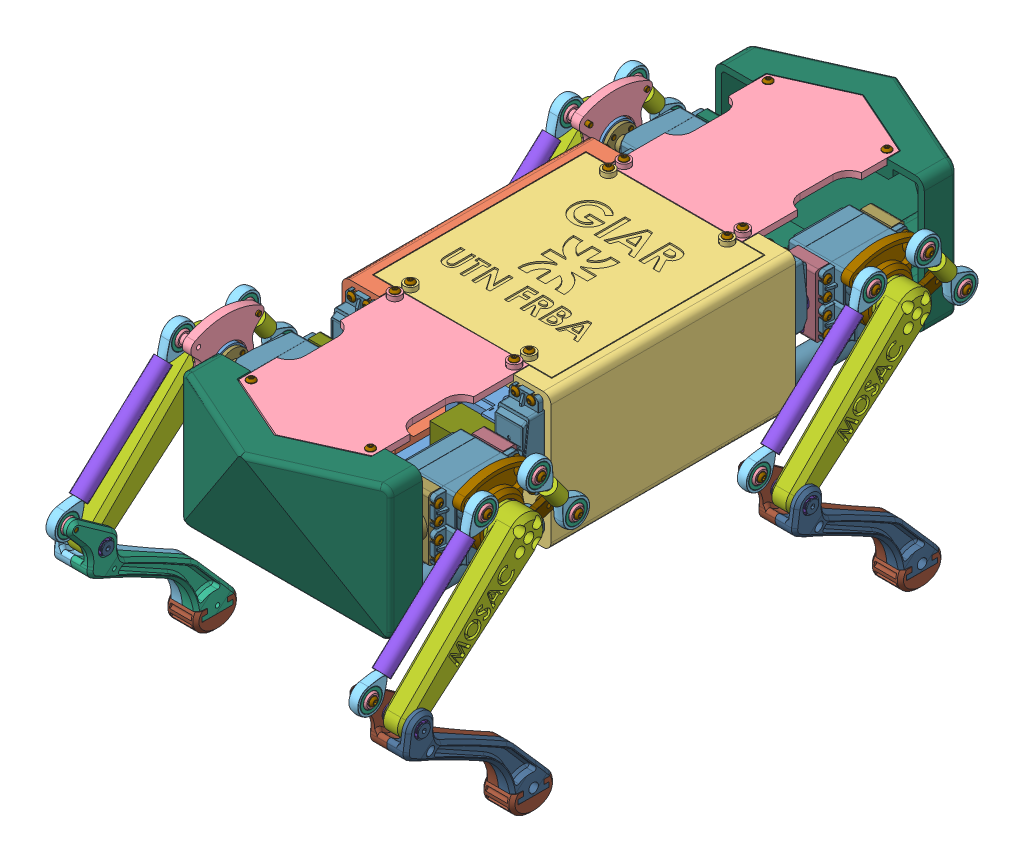
SolidWorks assembly Cuerpo_completo, configuration Default. Lengths in mm.
Overall size (654.71 199.05 461.18).
357 component instances, 69 part files, 170 mates.
Components (placement in the parent):
- Base-1: Base [Default] at (0 -43.5 0) size (85.5 47.11 157.51)
- Lateral_left-1: Lateral_left [Default] at (-45.25 0 0) x (-1 0 0) z (0 0 -1) size (34 87 157.5)
- Lateral_right-1: Lateral_right [Default] at (21.25 0 0) x (-1 0 0) z (0 0 -1) size (34 87 157.5)
- Extremidad_FL-1: Extremidad_FL [Default] at (10.785 83.987 4.7061) x (-1 0 0) z (0 0 -1) size (80.53 199.05 174.9)
  - Shoulder_Left-1: Shoulder_Left [Default] at (95.035 -70.5218 119.7561) x (0 -0.707107 -0.707107) z (1 0 0) size (47.5 48.5 9.25)
  - Tibia_Left-1: Tibia_Left [Default] at (96.6652 -236.7415 97.1828) size (25 98.84 110.57)
    - Tibia_left_1-1: Tibia_left_1 [Default] at (15.8698 98.4676 -50.9771) size (12.5 84.25 97.36)
    - Tibia_left_2-1: Tibia_left_2 [Default] at (15.8698 98.4676 -50.9771) size (12.5 98.84 110.57)
  - Femur-1: Femur [Left] at (105.035 -70.5218 119.7561) x (1 0 0) z (0 -0.735504 0.677521) size (23.66 120.1 24.2)
  - Ruleman_4x10x4-1: Ruleman_4x10x4 [Default] at (120.035 -138.2738 46.2057) x (0 0 1) z (-1 0 0) size (10 10 4)
  - Ruleman_4x10x4-2: Ruleman_4x10x4 [Default] at (105.035 -138.2738 46.2057) x (0 0 -1) z (1 0 0) size (10 10 4)
  - Tornillo_boton_M3-1: Tornillo_boton_M3 [12] at (119.185 -153.7137 52.4238) x (-1 0 0) z (0 0.029672 -0.99956) size (13.65 5.5 5.5)
  - Tornillo_fresado_4x12-1: Tornillo_fresado_4x12 [Default] at (98.755 -138.2738 46.2057) size (12 7.8 7.8)
  - Tornillo_fresado_4x12-2: Tornillo_fresado_4x12 [Default] at (126.315 -138.2738 46.2057) x (-1 0 0) z (0 0.011334 -0.999936) size (12 7.8 7.8)
  - Tornillo_boton_M3-2: Tornillo_boton_M3 [12] at (119.185 -209.0201 120.452) x (-1 0 0) z (0 -0.711874 -0.702307) size (13.65 5.5 5.5)
  - Tornillo_boton_M3-6: Tornillo_boton_M3 [15] at (113.935 -119.182 27.1139) x (-1 0 0) z (0 0.704901 -0.709306) size (16.65 5.5 5.5)
  - Paw-1: Paw [Default] at (112.535 -138.2738 46.2057) size (20.01 17.51 30.94)
  - Circular_horn-1: Circular_horn [Default] at (94.235 -70.5218 119.7561) x (0 -0.677521 -0.735504) z (1 0 0) size (20.6 20.6 5.5)
  - Ruleman_4x10x4-3: Ruleman_4x10x4 [Default] at (63.535 -80.787 160.3061) size (10 10 4)
  - Varilla_4mm-1: Varilla_4mm [Default] at (63.535 -80.787 156.3061) x (0.766791 0.641897 0) z (0 0 1) size (4 4 30)
  - DS3235-1: DS3235 [Default] at (65.785 -70.5218 129.7561) x (0 0 -1) z (0 -1 0) size (62.21 45.5 20.09)
  - DS3235-2: DS3235 [Default] at (65.785 -91.0521 129.7561) x (0 0 1) z (0 1 0) size (62.21 45.5 20.09)
  - DS3235-3: DS3235 [Default] at (63.535 -70.787 75.7061) x (0 -1 0) z (-1 0 0) size (62.21 45.5 20.09)
  - Holder_ball_bearing_side_left-4: Holder_ball_bearing_side_left [Default] at (63.535 -80.787 157.8061) size (20 40.56 10.5)
  - Holder_servo_side_left-2: Holder_servo_side_left [Default] at (63.535 -80.787 100.7061) x (1 0 0) z (0 0 -1) size (20 40.56 9)
  - Double_horn-2: Double_horn [Défaut] at (63.535 -80.787 103.2061) x (-1 0 0) z (0 0 -1) size (11.9 38 5)
  - 25T_horn-1: 25T_horn [Default] at (87.785 -91.0521 139.7561) x (0 -0.288263 -0.957551) z (0 -0.957551 0.288263) size (35.48 6.11 15.04)
  - Tornillo_boton_M3-13: Tornillo_boton_M3 [12] at (78.2777 -65.5218 154.5061) x (-1 0 0) z (0 -0.924225 -0.381849) size (13.65 5.5 5.5)
  - Tornillo_boton_M3-14: Tornillo_boton_M3 [12] at (78.2777 -75.5218 154.5061) x (-1 0 0) z (0 -0.85199 -0.523557) size (13.65 5.5 5.5)
  - Tornillo_boton_M3-16: Tornillo_boton_M3 [12] at (78.2777 -86.0521 154.5061) x (-1 0 0) z (0 -0.77839 -0.627782) size (13.65 5.5 5.5)
  - Tornillo_boton_M3-18: Tornillo_boton_M3 [12] at (78.2777 -96.0521 154.5061) x (-1 0 0) z (0 -0.716484 -0.697604) size (13.65 5.5 5.5)
  - Tornillo_boton_M3-20: Tornillo_boton_M3 [12] at (78.2777 -65.5218 105.0061) x (-1 0 0) z (0 -0.677445 -0.735574) size (13.65 5.5 5.5)
  - Tornillo_boton_M3-22: Tornillo_boton_M3 [12] at (78.2777 -75.5218 105.0061) x (-1 0 0) z (0 -0.670257 -0.742129) size (13.65 5.5 5.5)
  - Tornillo_boton_M3-24: Tornillo_boton_M3 [12] at (78.2777 -86.0521 105.0061) x (-1 0 0) z (0 -0.699933 -0.714209) size (13.65 5.5 5.5)
  - Tornillo_boton_M3-26: Tornillo_boton_M3 [12] at (78.2777 -96.0521 105.0061) x (-1 0 0) z (0 -0.763664 -0.645614) size (13.65 5.5 5.5)
  - Soporte_ruleman-1: Soporte_ruleman [Default] at (97.035 -70.5218 119.7561) x (0 0.735504 -0.677521) z (0 0.677521 0.735504) size (22.5 3 22.5)
  - Ruleman_6704-1: Ruleman_6704 [Default] at (97.035 -70.5218 119.7561) x (0 -1 0) z (0 0 1) size (27 4 27)
  - Tornillo_boton_M3-27: Tornillo_boton_M3 [20] at (112.885 -65.2371 125.493) x (-1 0 0) z (0 -0.924225 -0.381849) size (21.65 5.5 5.5)
  - Tornillo_boton_M3-28: Tornillo_boton_M3 [6] at (95.685 -70.5218 119.7561) x (-1 0 0) z (0 -0.924225 -0.381849) size (7.65 5.5 5.5)
  - Tornillo_boton_M3-29: Tornillo_boton_M3 [20] at (112.885 -64.7848 114.4714) x (-1 0 0) z (0 -0.85199 -0.523557) size (21.65 5.5 5.5)
  - Tornillo_boton_M3-30: Tornillo_boton_M3 [20] at (112.885 -75.8064 114.0192) x (-1 0 0) z (0 -0.77839 -0.627782) size (21.65 5.5 5.5)
  - Tornillo_boton_M3-31: Tornillo_boton_M3 [20] at (112.885 -76.2587 125.0408) x (-1 0 0) z (0 -0.716484 -0.697604) size (21.65 5.5 5.5)
  - Tuerca_3x0.5-1: Tuerca_3x0.5 [Default] at (93.885 -84.1338 162.7373) x (0 -1 0) z (0 0 1) size (5.5 2.3 6.35)
  - Tuerca_3x0.5-2: Tuerca_3x0.5 [Default] at (96.185 -84.1338 162.7373) x (0 -0.984981 -0.172664) z (0 -0.172664 0.984981) size (5.5 2.3 6.35)
  - Tuerca_3x0.5-5: Tuerca_3x0.5 [Default] at (98.485 -84.1338 162.7373) x (0 -0.965855 -0.259083) z (0 -0.259083 0.965855) size (5.5 2.3 6.35)
  - Tornillo_boton_M3-32: Tornillo_boton_M3 [20] at (110.435 -84.1338 162.7373) x (-1 0 0) z (0 -0.695492 -0.718534) size (21.65 5.5 5.5)
  - Tornillo_boton_M3-33: Tornillo_boton_M3 [20] at (113.935 -51.4299 100.6642) x (-1 0 0) z (0 -0.0053 -0.999986) size (21.65 5.5 5.5)
  - Tornillo_boton_M3-34: Tornillo_boton_M3 [15] at (110.435 -51.4299 138.848) x (-1 0 0) z (0 0.534452 -0.845199) size (16.65 5.5 5.5)
  - Rod_varilla_40.5mm-1: Rod_varilla_40.5mm [Default] at (104.785 -8.8899 107.9178) x (0 0.683874 0.7296) z (0 -0.7296 0.683874) size (28.74 19.93 60.72)
    - Rod M5-1: Rod M5 [Default] at (23.1289 -32.4219 37.6888) x (0.985148 -0.121869 0.120961) z (0.120961 0.992546 0.014852) size (19.76 42 17.66)
      - Ball_rod-1: Ball_rod [Default] at (-31.411 -18.0066 28.8086) x (-0.121869 0 0.992546) z (-0.992546 0 -0.121869) size (8 11.1 11.1)
      - Cuerpo_rod-1: Cuerpo_rod [20] at (-31.411 -51.0066 28.8086) x (0.121869 0 -0.992546) z (0.992546 0 0.121869) size (15.58 42 18)
      - Interfaz_rod-1: Interfaz_rod [Default] at (-31.411 -18.0066 28.8086) x (0.992546 0 0.121869) z (-0.121869 0 0.992546) size (14 14 6)
    - Rod M5-2: Rod M5 [Default] at (-41.1152 -32.4219 106.8885) x (-0.985148 -0.121869 -0.120961) z (-0.120961 0.992546 -0.014852) size (19.76 42 17.66)
      - Ball_rod-1: Ball_rod [Default] at (-31.411 -18.0066 28.8086) x (-0.121869 0 0.992546) z (-0.992546 0 -0.121869) size (8 11.1 11.1)
      - Cuerpo_rod-1: Cuerpo_rod [20] at (-31.411 -51.0066 28.8086) x (0.121869 0 -0.992546) z (0.992546 0 0.121869) size (15.58 42 18)
      - Interfaz_rod-1: Interfaz_rod [Default] at (-31.411 -18.0066 28.8086) x (0.992546 0 0.121869) z (-0.121869 0 0.992546) size (14 14 6)
    - Varilla_12mm-2: Varilla_12mm [Default] at (-9.7244 0 78.2439) x (0.985148 -0.121869 0.120961) z (0.120961 0.992546 0.014852) size (10 12 10)
  - Rod_varilla_100mm-1: Rod_varilla_100mm [Default] at (108.285 -114.4186 32.1131) x (0 0.647452 -0.762106) z (0 0.762106 0.647452) size (35.99 19.93 119.77)
    - Rod M5-1: Rod M5 [Default] at (30.3801 -32.4219 -21.3677) x (0.985148 -0.121869 0.120961) z (0.120961 0.992546 0.014852) size (19.76 42 17.66)
      - Ball_rod-1: Ball_rod [Default] at (-31.411 -18.0066 28.8086) x (-0.121869 0 0.992546) z (-0.992546 0 -0.121869) size (8 11.1 11.1)
      - Cuerpo_rod-1: Cuerpo_rod [20] at (-31.411 -51.0066 28.8086) x (0.121869 0 -0.992546) z (0.992546 0 0.121869) size (15.58 42 18)
      - Interfaz_rod-1: Interfaz_rod [Default] at (-31.411 -18.0066 28.8086) x (0.992546 0 0.121869) z (-0.121869 0 0.992546) size (14 14 6)
    - Rod M5-2: Rod M5 [Default] at (-41.1152 -32.4219 106.8885) x (-0.985148 -0.121869 -0.120961) z (-0.120961 0.992546 -0.014852) size (19.76 42 17.66)
      - Ball_rod-1: Ball_rod [Default] at (-31.411 -18.0066 28.8086) x (-0.121869 0 0.992546) z (-0.992546 0 -0.121869) size (8 11.1 11.1)
      - Cuerpo_rod-1: Cuerpo_rod [20] at (-31.411 -51.0066 28.8086) x (0.121869 0 -0.992546) z (0.992546 0 0.121869) size (15.58 42 18)
      - Interfaz_rod-1: Interfaz_rod [Default] at (-31.411 -18.0066 28.8086) x (0.992546 0 0.121869) z (-0.121869 0 0.992546) size (14 14 6)
    - Varilla_74mm-2: Varilla_74mm [Default] at (-9.8767 0 79.4846) x (0.985148 -0.121869 0.120961) z (0.120961 0.992546 0.014852) size (10 74 10)
  - Tornillo_boton_M3-36: Tornillo_boton_M3 [6] at (94.235 -91.0521 139.7561) x (-1 0 0) z (0 -0.85199 -0.523557) size (7.65 5.5 5.5)
  - Paw_simplificado-1: Paw_simplificado [Default] at (122.535 -206.2701 120.452) x (0 0.316293 -0.948662) z (0 0.948662 0.316293) size (34.5 20 34.5) (hidden)
- Extremidad_BL-1: Extremidad_BL [Default] at (10.785 83.987 254.8061) x (-1 0 0) z (0 0 -1) size (80.53 199.05 199.07)
  - Shoulder_Left-1: Shoulder_Left [Default] at (95.035 -70.5218 119.7561) x (0 -0.707107 -0.707107) z (1 0 0) size (47.5 48.5 9.25)
  - Tibia_Left-1: Tibia_Left [Default] at (96.6652 -236.7415 97.1828) size (25 98.84 110.57)
    - Tibia_left_1-1: Tibia_left_1 [Default] at (15.8698 98.4676 -50.9771) size (12.5 84.25 97.36)
    - Tibia_left_2-1: Tibia_left_2 [Default] at (15.8698 98.4676 -50.9771) size (12.5 98.84 110.57)
  - Femur-1: Femur [Left] at (105.035 -70.5218 119.7561) x (1 0 0) z (0 -0.735504 0.677521) size (23.66 120.1 24.2)
  - Ruleman_4x10x4-1: Ruleman_4x10x4 [Default] at (120.035 -138.2738 46.2057) x (0 0 1) z (-1 0 0) size (10 10 4)
  - Ruleman_4x10x4-2: Ruleman_4x10x4 [Default] at (105.035 -138.2738 46.2057) x (0 0 -1) z (1 0 0) size (10 10 4)
  - Tornillo_boton_M3-1: Tornillo_boton_M3 [12] at (119.185 -153.7137 52.4238) x (-1 0 0) z (0 0.029672 -0.99956) size (13.65 5.5 5.5)
  - Tornillo_fresado_4x12-1: Tornillo_fresado_4x12 [Default] at (98.755 -138.2738 46.2057) size (12 7.8 7.8)
  - Tornillo_fresado_4x12-2: Tornillo_fresado_4x12 [Default] at (126.315 -138.2738 46.2057) x (-1 0 0) z (0 0.011334 -0.999936) size (12 7.8 7.8)
  - Tornillo_boton_M3-2: Tornillo_boton_M3 [12] at (119.185 -209.0201 120.452) x (-1 0 0) z (0 -0.711874 -0.702307) size (13.65 5.5 5.5)
  - Tornillo_boton_M3-6: Tornillo_boton_M3 [12] at (113.935 -119.182 27.1139) x (-1 0 0) z (0 -0.964026 -0.265809) size (13.65 5.5 5.5)
  - Tornillo_boton_M3-8: Tornillo_boton_M3 [15] at (110.435 -51.4299 138.848) x (-1 0 0) z (0 0.876345 -0.481683) size (16.65 5.5 5.5)
  - Tornillo_boton_M3-10: Tornillo_boton_M3 [15] at (113.935 -51.4299 100.6642) x (-1 0 0) z (0 0.538918 -0.842358) size (16.65 5.5 5.5)
  - Tornillo_boton_M3-12: Tornillo_boton_M3 [20] at (110.435 -84.1338 162.7373) x (-1 0 0) z (0 -0.467279 -0.88411) size (21.65 5.5 5.5)
  - Paw-1: Paw [Default] at (112.535 -138.2738 46.2057) size (20.01 17.51 30.94)
  - Circular_horn-1: Circular_horn [Default] at (94.235 -70.5218 119.7561) x (0 -0.677521 -0.735504) z (1 0 0) size (20.6 20.6 5.5)
  - Ruleman_4x10x4-3: Ruleman_4x10x4 [Default] at (63.535 -80.787 99.2061) x (0.923728 0.383049 0) z (0 0 -1) size (10 10 4)
  - Varilla_4mm-1: Varilla_4mm [Default] at (63.535 -80.787 103.2061) x (0.954184 -0.29922 0) z (0 0 -1) size (4 4 30)
  - DS3235-1: DS3235 [Default] at (65.785 -70.5218 129.7561) x (0 0 -1) z (0 -1 0) size (62.21 45.5 20.09)
  - DS3235-2: DS3235 [Default] at (65.785 -91.0521 129.7561) x (0 0 1) z (0 1 0) size (62.21 45.5 20.09)
  - DS3235-3: DS3235 [Default] at (63.535 -70.787 183.8061) x (0 -1 0) z (1 0 0) size (62.21 45.5 20.09)
  - Holder_ball_bearing_side_left-4: Holder_ball_bearing_side_left [Default] at (63.535 -80.787 101.7061) x (1 0 0) z (0 0 -1) size (20 40.56 10.5)
  - Holder_servo_side_left-2: Holder_servo_side_left [Default] at (63.535 -80.787 158.8061) size (20 40.56 9)
  - Double_horn-2: Double_horn [Défaut] at (63.535 -80.787 156.3061) x (-1 0 0) z (0 0 1) size (11.9 38 5)
  - 25T_horn-1: 25T_horn [Default] at (87.785 -91.0521 139.7561) x (0 -0.288263 -0.957551) z (0 -0.957551 0.288263) size (35.48 6.11 15.04)
  - Tornillo_boton_M3-13: Tornillo_boton_M3 [12] at (78.2777 -65.5218 154.5061) x (-1 0 0) z (0 -0.924225 -0.381849) size (13.65 5.5 5.5)
  - Tornillo_boton_M3-14: Tornillo_boton_M3 [12] at (78.2777 -75.5218 154.5061) x (-1 0 0) z (0 -0.85199 -0.523557) size (13.65 5.5 5.5)
  - Tornillo_boton_M3-16: Tornillo_boton_M3 [12] at (78.2777 -86.0521 154.5061) x (-1 0 0) z (0 -0.77839 -0.627782) size (13.65 5.5 5.5)
  - Tornillo_boton_M3-18: Tornillo_boton_M3 [12] at (78.2777 -96.0521 154.5061) x (-1 0 0) z (0 -0.716484 -0.697604) size (13.65 5.5 5.5)
  - Tornillo_boton_M3-20: Tornillo_boton_M3 [12] at (78.2777 -65.5218 105.0061) x (-1 0 0) z (0 -0.677445 -0.735574) size (13.65 5.5 5.5)
  - Tornillo_boton_M3-22: Tornillo_boton_M3 [12] at (78.2777 -75.5218 105.0061) x (-1 0 0) z (0 -0.670257 -0.742129) size (13.65 5.5 5.5)
  - Tornillo_boton_M3-24: Tornillo_boton_M3 [12] at (78.2777 -86.0521 105.0061) x (-1 0 0) z (0 -0.699933 -0.714209) size (13.65 5.5 5.5)
  - Tornillo_boton_M3-26: Tornillo_boton_M3 [12] at (78.2777 -96.0521 105.0061) x (-1 0 0) z (0 -0.763664 -0.645614) size (13.65 5.5 5.5)
  - Ruleman_6704-1: Ruleman_6704 [Default] at (97.035 -70.5218 119.7561) x (0 -1 0) z (0 0 1) size (27 4 27)
  - Soporte_ruleman-1: Soporte_ruleman [Default] at (97.035 -70.5218 119.7561) x (0 0.735504 -0.677521) z (0 0.677521 0.735504) size (22.5 3 22.5)
  - Tornillo_boton_M3-28: Tornillo_boton_M3 [20] at (112.885 -65.2371 125.493) x (-1 0 0) z (0 0.924225 0.381849) size (21.65 5.5 5.5)
  - Tornillo_boton_M3-29: Tornillo_boton_M3 [20] at (112.885 -64.7848 114.4714) x (-1 0 0) z (0 0.85199 0.523557) size (21.65 5.5 5.5)
  - Tornillo_boton_M3-31: Tornillo_boton_M3 [20] at (112.885 -75.8064 114.0192) x (-1 0 0) z (0 0.77839 0.627782) size (21.65 5.5 5.5)
  - Tornillo_boton_M3-33: Tornillo_boton_M3 [20] at (112.885 -76.2587 125.0408) x (-1 0 0) z (0 0.716484 0.697604) size (21.65 5.5 5.5)
  - Tornillo_boton_M3-35: Tornillo_boton_M3 [6] at (95.685 -70.5218 119.7561) x (-1 0 0) z (0 0.230333 0.973112) size (7.65 5.5 5.5)
  - Tuerca_3x0.5-1: Tuerca_3x0.5 [Default] at (93.885 -84.1338 162.7373) x (0 -1 0) z (0 0 1) size (5.5 2.3 6.35)
  - Tuerca_3x0.5-2: Tuerca_3x0.5 [Default] at (96.185 -84.1338 162.7373) x (0 -0.987351 -0.158553) z (0 -0.158553 0.987351) size (5.5 2.3 6.35)
  - Tuerca_3x0.5-3: Tuerca_3x0.5 [Default] at (98.485 -84.1338 162.7373) x (0 -0.959125 -0.282984) z (0 -0.282984 0.959125) size (5.5 2.3 6.35)
  - Rod_varilla_100mm-1: Rod_varilla_100mm [Default] at (108.285 -114.5898 32.2708) x (0 -0.81259 0.582835) z (0 0.582835 0.81259) size (35.99 19.93 119.77)
    - Rod M5-1: Rod M5 [Default] at (30.3801 -32.4219 -21.3677) x (0.985148 -0.121869 0.120961) z (0.120961 0.992546 0.014852) size (19.76 42 17.66)
      - Ball_rod-1: Ball_rod [Default] at (-31.411 -18.0066 28.8086) x (-0.121869 0 0.992546) z (-0.992546 0 -0.121869) size (8 11.1 11.1)
      - Cuerpo_rod-1: Cuerpo_rod [20] at (-31.411 -51.0066 28.8086) x (0.121869 0 -0.992546) z (0.992546 0 0.121869) size (15.58 42 18)
      - Interfaz_rod-1: Interfaz_rod [Default] at (-31.411 -18.0066 28.8086) x (0.992546 0 0.121869) z (-0.121869 0 0.992546) size (14 14 6)
    - Rod M5-2: Rod M5 [Default] at (-41.1152 -32.4219 106.8885) x (-0.985148 -0.121869 -0.120961) z (-0.120961 0.992546 -0.014852) size (19.76 42 17.66)
      - Ball_rod-1: Ball_rod [Default] at (-31.411 -18.0066 28.8086) x (-0.121869 0 0.992546) z (-0.992546 0 -0.121869) size (8 11.1 11.1)
      - Cuerpo_rod-1: Cuerpo_rod [20] at (-31.411 -51.0066 28.8086) x (0.121869 0 -0.992546) z (0.992546 0 0.121869) size (15.58 42 18)
      - Interfaz_rod-1: Interfaz_rod [Default] at (-31.411 -18.0066 28.8086) x (0.992546 0 0.121869) z (-0.121869 0 0.992546) size (14 14 6)
    - Varilla_74mm-2: Varilla_74mm [Default] at (-9.8767 0 79.4846) x (0.985148 -0.121869 0.120961) z (0.120961 0.992546 0.014852) size (10 74 10)
  - Rod_varilla_40.5mm-1: Rod_varilla_40.5mm [Default] at (104.785 -8.8899 107.9178) x (0 0.683874 0.7296) z (0 -0.7296 0.683874) size (28.74 19.93 60.72)
    - Rod M5-1: Rod M5 [Default] at (23.1289 -32.4219 37.6888) x (0.985148 -0.121869 0.120961) z (0.120961 0.992546 0.014852) size (19.76 42 17.66)
      - Ball_rod-1: Ball_rod [Default] at (-31.411 -18.0066 28.8086) x (-0.121869 0 0.992546) z (-0.992546 0 -0.121869) size (8 11.1 11.1)
      - Cuerpo_rod-1: Cuerpo_rod [20] at (-31.411 -51.0066 28.8086) x (0.121869 0 -0.992546) z (0.992546 0 0.121869) size (15.58 42 18)
      - Interfaz_rod-1: Interfaz_rod [Default] at (-31.411 -18.0066 28.8086) x (0.992546 0 0.121869) z (-0.121869 0 0.992546) size (14 14 6)
    - Rod M5-2: Rod M5 [Default] at (-41.1152 -32.4219 106.8885) x (-0.985148 -0.121869 -0.120961) z (-0.120961 0.992546 -0.014852) size (19.76 42 17.66)
      - Ball_rod-1: Ball_rod [Default] at (-31.411 -18.0066 28.8086) x (-0.121869 0 0.992546) z (-0.992546 0 -0.121869) size (8 11.1 11.1)
      - Cuerpo_rod-1: Cuerpo_rod [20] at (-31.411 -51.0066 28.8086) x (0.121869 0 -0.992546) z (0.992546 0 0.121869) size (15.58 42 18)
      - Interfaz_rod-1: Interfaz_rod [Default] at (-31.411 -18.0066 28.8086) x (0.992546 0 0.121869) z (-0.121869 0 0.992546) size (14 14 6)
    - Varilla_12mm-2: Varilla_12mm [Default] at (-9.7244 0 78.2439) x (0.985148 -0.121869 0.120961) z (0.120961 0.992546 0.014852) size (10 12 10)
  - Tornillo_boton_M3-36: Tornillo_boton_M3 [6] at (94.235 -91.0521 139.7561) x (-1 0 0) z (0 0.073129 0.997322) size (7.65 5.5 5.5)
- Extremidad_FR-2: Extremidad_FR [Default] at (34.5568 -196.6228 -200.4391) x (-1 0 0) z (0 0 -1) size (80.53 199.05 181.57)
  - Femur-1: Femur [Right] at (-59.6932 210.088 -85.3891) x (-1 0 0) z (0 0.735504 -0.677521) size (23.66 120.1 24.2)
  - Shoulder_Right-1: Shoulder_Right [Default] at (-65.9932 210.088 -85.3891) x (0 -0.707107 -0.707107) z (1 0 0) size (47.5 48.5 9.25)
  - Tibia_right-1: Tibia_right [Default] at (-64.8358 52.2502 -218.3849) size (25 98.84 110.57)
    - Tibia_right_1-1: Tibia_right_1 [Default] at (-2.3574 90.0857 59.4454) size (12.5 84.25 99.27)
    - Tibia_right_2-1: Tibia_right_2 [Default] at (-2.3574 90.0857 59.4454) size (12.5 98.84 110.57)
  - Paw-1: Paw [Default] at (-67.1932 142.3359 -158.9395) size (20.01 17.51 30.94)
  - Ruleman_4x10x4-1: Ruleman_4x10x4 [Default] at (-18.1932 199.8228 -44.8391) size (10 10 4)
  - Varilla_4mm-1: Varilla_4mm [Default] at (-18.1932 199.8228 -48.8391) size (4 4 30)
  - Holder_ball_bearing_side_right-1: Holder_ball_bearing_side_right [Default] at (-18.1932 199.8228 -63.3391) x (-1 0 0) z (0 0 -1) size (20 40.56 10.5)
  - Holder_servo_side_right-1: Holder_servo_side_right [Default] at (-18.1932 199.8228 -86.4391) x (-1 0 0) z (0 0 1) size (20 40.56 9)
  - DS3235-1: DS3235 [Default] at (-20.4432 189.5576 -75.3891) x (0 0 1) z (0 -1 0) size (62.21 45.5 20.09)
  - DS3235-2: DS3235 [Default] at (-20.4432 210.088 -75.3891) x (0 0 -1) z (0 1 0) size (62.21 45.5 20.09)
  - DS3235-3: DS3235 [Default] at (-18.1932 209.8228 -129.4391) x (0 -1 0) z (-1 0 0) size (62.21 45.5 20.09)
  - Double_horn-1: Double_horn [Défaut] at (-18.1932 199.8228 -101.9391) x (-1 0 0) z (0 0 -1) size (11.9 38 5)
  - Circular_horn-1: Circular_horn [Default] at (-48.8932 210.088 -85.3891) x (0 0.735504 -0.677521) z (-1 0 0) size (20.6 20.6 5.5)
  - Tornillo_boton_M3-1: Tornillo_boton_M3 [6] at (-50.3432 210.088 -85.3891) size (7.65 5.5 5.5)
  - 25T_horn-1: 25T_horn [Default] at (-42.4432 189.5576 -65.3891) x (0 -0.288263 -0.957551) z (0 0.957551 -0.288263) size (35.48 6.11 15.04)
  - Ruleman_4x10x4-2: Ruleman_4x10x4 [Default] at (-74.6932 142.3359 -158.9395) x (0 0 -1) z (1 0 0) size (10 10 4)
  - Ruleman_4x10x4-3: Ruleman_4x10x4 [Default] at (-59.6932 142.3359 -158.9395) x (0 0 1) z (-1 0 0) size (10 10 4)
  - Tornillo_fresado_4x12-1: Tornillo_fresado_4x12 [Default] at (-53.4132 142.3359 -158.9395) x (-1 0 0) z (0 -0.924225 -0.381849) size (12 7.8 7.8)
  - Tornillo_fresado_4x12-2: Tornillo_fresado_4x12 [Default] at (-80.9732 142.3359 -158.9395) size (12 7.8 7.8)
  - Tornillo_boton_M3-2: Tornillo_boton_M3 [12] at (-73.8432 126.8961 -152.7214) size (13.65 5.5 5.5)
  - Tornillo_boton_M3-3: Tornillo_boton_M3 [12] at (-73.8432 71.5897 -84.6932) x (1 0 0) z (0 -0.158553 0.987351) size (13.65 5.5 5.5)
  - Tornillo_boton_M3-4: Tornillo_boton_M3 [12] at (-68.5932 161.4278 -178.0313) x (1 0 0) z (0 -0.158553 0.987351) size (13.65 5.5 5.5)
  - Tornillo_boton_M3-6: Tornillo_boton_M3 [15] at (-68.5932 229.1799 -104.481) x (1 0 0) z (0 -0.546764 0.837287) size (16.65 5.5 5.5)
  - Tornillo_boton_M3-8: Tornillo_boton_M3 [15] at (-65.0932 229.1799 -66.2972) x (1 0 0) z (0 0.773734 0.633511) size (16.65 5.5 5.5)
  - Tornillo_boton_M3-10: Tornillo_boton_M3 [20] at (-65.0932 196.4759 -42.4079) x (1 0 0) z (0 0.999802 0.019924) size (21.65 5.5 5.5)
  - Tornillo_boton_M3-11: Tornillo_boton_M3 [12] at (-32.9359 215.088 -50.6391) size (13.65 5.5 5.5)
  - Tornillo_boton_M3-12: Tornillo_boton_M3 [12] at (-32.9359 205.088 -50.6391) x (1 0 0) z (0 -0.158553 0.987351) size (13.65 5.5 5.5)
  - Tornillo_boton_M3-14: Tornillo_boton_M3 [12] at (-32.9359 194.5576 -50.6391) x (1 0 0) z (0 -0.282984 0.959125) size (13.65 5.5 5.5)
  - Tornillo_boton_M3-16: Tornillo_boton_M3 [12] at (-32.9359 184.5576 -50.6391) x (1 0 0) z (0 -0.371154 0.928571) size (13.65 5.5 5.5)
  - Tornillo_boton_M3-18: Tornillo_boton_M3 [12] at (-32.9359 215.088 -100.1391) x (1 0 0) z (0 -0.421154 0.906989) size (13.65 5.5 5.5)
  - Tornillo_boton_M3-20: Tornillo_boton_M3 [12] at (-32.9359 205.088 -100.1391) x (1 0 0) z (0 -0.429957 0.902849) size (13.65 5.5 5.5)
  - Tornillo_boton_M3-22: Tornillo_boton_M3 [12] at (-32.9359 194.5576 -100.1391) x (1 0 0) z (0 -0.39282 0.919615) size (13.65 5.5 5.5)
  - Tornillo_boton_M3-24: Tornillo_boton_M3 [12] at (-32.9359 184.5576 -100.1391) x (1 0 0) z (0 -0.305088 0.952324) size (13.65 5.5 5.5)
  - Ruleman_6704-1: Ruleman_6704 [Default] at (-51.6932 210.088 -85.3891) x (0 1 0) z (0 0 1) size (27 4 27)
  - Soporte_ruleman-1: Soporte_ruleman [Default] at (-48.6932 210.088 -85.3891) x (0 0.677521 0.735504) z (0 -0.735504 0.677521) size (22.5 3 22.5)
  - Tornillo_boton_M3-25: Tornillo_boton_M3 [20] at (-67.5432 215.3726 -79.6522) size (21.65 5.5 5.5)
  - Tornillo_boton_M3-26: Tornillo_boton_M3 [20] at (-67.5432 215.8249 -90.6738) x (1 0 0) z (0 -0.158553 0.987351) size (21.65 5.5 5.5)
  - Tornillo_boton_M3-28: Tornillo_boton_M3 [20] at (-67.5432 204.8033 -91.126) x (1 0 0) z (0 -0.282984 0.959125) size (21.65 5.5 5.5)
  - Tornillo_boton_M3-30: Tornillo_boton_M3 [20] at (-67.5432 204.3511 -80.1044) x (1 0 0) z (0 -0.371154 0.928571) size (21.65 5.5 5.5)
  - Tuerca_3x0.5-1: Tuerca_3x0.5 [Default] at (-48.5432 196.4759 -42.4079) x (0 1 0) z (0 0 1) size (5.5 2.3 6.35)
  - Tuerca_3x0.5-2: Tuerca_3x0.5 [Default] at (-50.8432 196.4759 -42.4079) x (0 0.987351 0.158553) z (0 -0.158553 0.987351) size (5.5 2.3 6.35)
  - Tuerca_3x0.5-3: Tuerca_3x0.5 [Default] at (-53.1432 196.4759 -42.4079) x (0 0.959125 0.282984) z (0 -0.282984 0.959125) size (5.5 2.3 6.35)
  - Tornillo_boton_M3-31: Tornillo_boton_M3 [6] at (-48.8932 189.5576 -65.3891) x (1 0 0) z (0 -0.158553 0.987351) size (7.65 5.5 5.5)
  - Rod_varilla_100mm-1: Rod_varilla_100mm [Default] at (-62.9432 166.0199 -172.8744) x (0 -0.81259 0.582835) z (0 0.582835 0.81259) size (35.99 19.93 119.77)
    - Rod M5-1: Rod M5 [Default] at (30.3801 -32.4219 -21.3677) x (0.985148 -0.121869 0.120961) z (0.120961 0.992546 0.014852) size (19.76 42 17.66)
      - Ball_rod-1: Ball_rod [Default] at (-31.411 -18.0066 28.8086) x (-0.121869 0 0.992546) z (-0.992546 0 -0.121869) size (8 11.1 11.1)
      - Cuerpo_rod-1: Cuerpo_rod [20] at (-31.411 -51.0066 28.8086) x (0.121869 0 -0.992546) z (0.992546 0 0.121869) size (15.58 42 18)
      - Interfaz_rod-1: Interfaz_rod [Default] at (-31.411 -18.0066 28.8086) x (0.992546 0 0.121869) z (-0.121869 0 0.992546) size (14 14 6)
    - Rod M5-2: Rod M5 [Default] at (-41.1152 -32.4219 106.8885) x (-0.985148 -0.121869 -0.120961) z (-0.120961 0.992546 -0.014852) size (19.76 42 17.66)
      - Ball_rod-1: Ball_rod [Default] at (-31.411 -18.0066 28.8086) x (-0.121869 0 0.992546) z (-0.992546 0 -0.121869) size (8 11.1 11.1)
      - Cuerpo_rod-1: Cuerpo_rod [20] at (-31.411 -51.0066 28.8086) x (0.121869 0 -0.992546) z (0.992546 0 0.121869) size (15.58 42 18)
      - Interfaz_rod-1: Interfaz_rod [Default] at (-31.411 -18.0066 28.8086) x (0.992546 0 0.121869) z (-0.121869 0 0.992546) size (14 14 6)
    - Varilla_74mm-2: Varilla_74mm [Default] at (-9.8767 0 79.4846) x (0.985148 -0.121869 0.120961) z (0.120961 0.992546 0.014852) size (10 74 10)
  - Rod_varilla_40.5mm-1: Rod_varilla_40.5mm [Default] at (-59.4432 271.5826 -97.4154) x (0 -0.487054 -0.873372) z (0 -0.873372 0.487054) size (28.74 19.93 60.72)
    - Rod M5-1: Rod M5 [Default] at (23.1289 -32.4219 37.6888) x (0.985148 -0.121869 0.120961) z (0.120961 0.992546 0.014852) size (19.76 42 17.66)
      - Ball_rod-1: Ball_rod [Default] at (-31.411 -18.0066 28.8086) x (-0.121869 0 0.992546) z (-0.992546 0 -0.121869) size (8 11.1 11.1)
      - Cuerpo_rod-1: Cuerpo_rod [20] at (-31.411 -51.0066 28.8086) x (0.121869 0 -0.992546) z (0.992546 0 0.121869) size (15.58 42 18)
      - Interfaz_rod-1: Interfaz_rod [Default] at (-31.411 -18.0066 28.8086) x (0.992546 0 0.121869) z (-0.121869 0 0.992546) size (14 14 6)
    - Rod M5-2: Rod M5 [Default] at (-41.1152 -32.4219 106.8885) x (-0.985148 -0.121869 -0.120961) z (-0.120961 0.992546 -0.014852) size (19.76 42 17.66)
      - Ball_rod-1: Ball_rod [Default] at (-31.411 -18.0066 28.8086) x (-0.121869 0 0.992546) z (-0.992546 0 -0.121869) size (8 11.1 11.1)
      - Cuerpo_rod-1: Cuerpo_rod [20] at (-31.411 -51.0066 28.8086) x (0.121869 0 -0.992546) z (0.992546 0 0.121869) size (15.58 42 18)
      - Interfaz_rod-1: Interfaz_rod [Default] at (-31.411 -18.0066 28.8086) x (0.992546 0 0.121869) z (-0.121869 0 0.992546) size (14 14 6)
    - Varilla_12mm-2: Varilla_12mm [Default] at (-9.7244 0 78.2439) x (0.985148 -0.121869 0.120961) z (0.120961 0.992546 0.014852) size (10 12 10)
- Extremidad_BR-1: Extremidad_BR [Default] at (35.81 -209.5088 12.3834) x (-1 0 0) z (0 0 -1) size (80.53 199.05 199.07)
  - Femur-1: Femur [Right] at (-58.44 222.974 -122.6666) x (-1 0 0) z (0 0.735504 -0.677521) size (23.66 120.1 24.2)
  - Shoulder_Right-1: Shoulder_Right [Default] at (-64.74 222.974 -122.6666) x (0 -0.707107 -0.707107) z (1 0 0) size (47.5 48.5 9.25)
  - Tibia_right-1: Tibia_right [Default] at (-63.5826 65.1363 -255.6624) size (25 98.84 110.57)
    - Tibia_right_1-1: Tibia_right_1 [Default] at (-2.3574 90.0857 59.4454) size (12.5 84.25 99.27)
    - Tibia_right_2-1: Tibia_right_2 [Default] at (-2.3574 90.0857 59.4454) size (12.5 98.84 110.57)
  - Paw-1: Paw [Default] at (-65.94 155.2219 -196.217) size (20.01 17.51 30.94)
  - Ruleman_4x10x4-1: Ruleman_4x10x4 [Default] at (-16.94 212.7088 -143.2166) x (0.923728 0.383049 0) z (0 0 -1) size (10 10 4)
  - Varilla_4mm-1: Varilla_4mm [Default] at (-16.94 212.7088 -139.2166) x (0.923728 0.383049 0) z (0 0 -1) size (4 4 30)
  - Holder_ball_bearing_side_right-1: Holder_ball_bearing_side_right [Default] at (-16.94 212.7088 -124.7166) x (-1 0 0) z (0 0 1) size (20 40.56 10.5)
  - Holder_servo_side_right-1: Holder_servo_side_right [Default] at (-16.94 212.7088 -101.6166) x (-1 0 0) z (0 0 -1) size (20 40.56 9)
  - DS3235-1: DS3235 [Default] at (-19.19 202.4436 -112.6666) x (0 0 1) z (0 -1 0) size (62.21 45.5 20.09)
  - DS3235-2: DS3235 [Default] at (-19.19 222.974 -112.6666) x (0 0 -1) z (0 1 0) size (62.21 45.5 20.09)
  - DS3235-3: DS3235 [Default] at (-16.94 222.7088 -58.6166) x (0 -1 0) z (1 0 0) size (62.21 45.5 20.09)
  - Double_horn-1: Double_horn [Défaut] at (-16.94 212.7088 -86.1166) x (-1 0 0) z (0 0 1) size (11.9 38 5)
  - Circular_horn-1: Circular_horn [Default] at (-47.64 222.974 -122.6666) x (0 -0.735504 0.677521) z (-1 0 0) size (20.6 20.6 5.5)
  - Tornillo_boton_M3-1: Tornillo_boton_M3 [6] at (-49.09 222.974 -122.6666) size (7.65 5.5 5.5)
  - 25T_horn-1: 25T_horn [Default] at (-41.19 202.4436 -102.6666) x (0 -0.288263 -0.957551) z (0 0.957551 -0.288263) size (35.48 6.11 15.04)
  - Ruleman_4x10x4-2: Ruleman_4x10x4 [Default] at (-73.44 155.2219 -196.217) x (0 0 -1) z (1 0 0) size (10 10 4)
  - Ruleman_4x10x4-3: Ruleman_4x10x4 [Default] at (-58.44 155.2219 -196.217) x (0 0 1) z (-1 0 0) size (10 10 4)
  - Tornillo_fresado_4x12-1: Tornillo_fresado_4x12 [Default] at (-52.16 155.2219 -196.217) x (-1 0 0) z (0 -0.924225 -0.381849) size (12 7.8 7.8)
  - Tornillo_fresado_4x12-2: Tornillo_fresado_4x12 [Default] at (-79.72 155.2219 -196.217) size (12 7.8 7.8)
  - Tornillo_boton_M3-2: Tornillo_boton_M3 [12] at (-72.59 139.7821 -189.9989) size (13.65 5.5 5.5)
  - Tornillo_boton_M3-3: Tornillo_boton_M3 [12] at (-72.59 84.4757 -121.9708) x (1 0 0) z (0 -0.158553 0.987351) size (13.65 5.5 5.5)
  - Tornillo_boton_M3-4: Tornillo_boton_M3 [12] at (-67.34 174.3138 -215.3089) x (1 0 0) z (0 -0.158553 0.987351) size (13.65 5.5 5.5)
  - Tornillo_boton_M3-6: Tornillo_boton_M3 [15] at (-67.34 242.0659 -141.7585) x (1 0 0) z (0 -0.282984 0.959125) size (16.65 5.5 5.5)
  - Tornillo_boton_M3-8: Tornillo_boton_M3 [15] at (-63.84 242.0659 -103.5748) x (1 0 0) z (0 -0.371154 0.928571) size (16.65 5.5 5.5)
  - Tornillo_boton_M3-10: Tornillo_boton_M3 [20] at (-63.84 209.3619 -79.6854) x (1 0 0) z (0 -0.401747 0.915751) size (21.65 5.5 5.5)
  - Tornillo_boton_M3-11: Tornillo_boton_M3 [12] at (-31.6827 227.974 -87.9166) size (13.65 5.5 5.5)
  - Tornillo_boton_M3-12: Tornillo_boton_M3 [12] at (-31.6827 217.974 -87.9166) x (1 0 0) z (0 -0.158553 0.987351) size (13.65 5.5 5.5)
  - Tornillo_boton_M3-14: Tornillo_boton_M3 [12] at (-31.6827 207.4436 -87.9166) x (1 0 0) z (0 -0.282984 0.959125) size (13.65 5.5 5.5)
  - Tornillo_boton_M3-16: Tornillo_boton_M3 [12] at (-31.6827 197.4436 -87.9166) x (1 0 0) z (0 -0.371154 0.928571) size (13.65 5.5 5.5)
  - Tornillo_boton_M3-18: Tornillo_boton_M3 [12] at (-31.6827 227.974 -137.4166) x (1 0 0) z (0 -0.421154 0.906989) size (13.65 5.5 5.5)
  - Tornillo_boton_M3-20: Tornillo_boton_M3 [12] at (-31.6827 217.974 -137.4166) x (1 0 0) z (0 -0.429957 0.902849) size (13.65 5.5 5.5)
  - Tornillo_boton_M3-22: Tornillo_boton_M3 [12] at (-31.6827 207.4436 -137.4166) x (1 0 0) z (0 -0.39282 0.919615) size (13.65 5.5 5.5)
  - Tornillo_boton_M3-24: Tornillo_boton_M3 [12] at (-31.6827 197.4436 -137.4166) x (1 0 0) z (0 -0.305088 0.952324) size (13.65 5.5 5.5)
  - Soporte_ruleman-1: Soporte_ruleman [Default] at (-50.44 222.974 -122.6666) x (0 -0.677521 -0.735504) z (0 -0.735504 0.677521) size (22.5 3 22.5)
  - Ruleman_6704-1: Ruleman_6704 [Default] at (-50.44 222.974 -122.6666) x (0 1 0) z (0 0 1) size (27 4 27)
  - Tornillo_boton_M3-25: Tornillo_boton_M3 [20] at (-66.29 228.2587 -116.9297) size (21.65 5.5 5.5)
  - Tornillo_boton_M3-26: Tornillo_boton_M3 [20] at (-66.29 228.7109 -127.9513) x (1 0 0) z (0 -0.158553 0.987351) size (21.65 5.5 5.5)
  - Tornillo_boton_M3-28: Tornillo_boton_M3 [20] at (-66.29 217.6893 -128.4036) x (1 0 0) z (0 -0.282984 0.959125) size (21.65 5.5 5.5)
  - Tornillo_boton_M3-30: Tornillo_boton_M3 [20] at (-66.29 217.2371 -117.382) x (1 0 0) z (0 -0.371154 0.928571) size (21.65 5.5 5.5)
  - Tuerca_3x0.5-1: Tuerca_3x0.5 [Default] at (-47.29 209.3619 -79.6854) x (0 1 0) z (0 0 1) size (5.5 2.3 6.35)
  - Tuerca_3x0.5-2: Tuerca_3x0.5 [Default] at (-49.59 209.3619 -79.6854) x (0 0.987351 0.158553) z (0 -0.158553 0.987351) size (5.5 2.3 6.35)
  - Tuerca_3x0.5-3: Tuerca_3x0.5 [Default] at (-51.89 209.3619 -79.6854) x (0 0.959125 0.282984) z (0 -0.282984 0.959125) size (5.5 2.3 6.35)
  - Rod_varilla_100mm-1: Rod_varilla_100mm [Default] at (-61.69 178.906 -210.152) x (0 -0.81259 0.582835) z (0 0.582835 0.81259) size (35.99 19.93 119.77)
    - Rod M5-1: Rod M5 [Default] at (30.3801 -32.4219 -21.3677) x (0.985148 -0.121869 0.120961) z (0.120961 0.992546 0.014852) size (19.76 42 17.66)
      - Ball_rod-1: Ball_rod [Default] at (-31.411 -18.0066 28.8086) x (-0.121869 0 0.992546) z (-0.992546 0 -0.121869) size (8 11.1 11.1)
      - Cuerpo_rod-1: Cuerpo_rod [20] at (-31.411 -51.0066 28.8086) x (0.121869 0 -0.992546) z (0.992546 0 0.121869) size (15.58 42 18)
      - Interfaz_rod-1: Interfaz_rod [Default] at (-31.411 -18.0066 28.8086) x (0.992546 0 0.121869) z (-0.121869 0 0.992546) size (14 14 6)
    - Rod M5-2: Rod M5 [Default] at (-41.1152 -32.4219 106.8885) x (-0.985148 -0.121869 -0.120961) z (-0.120961 0.992546 -0.014852) size (19.76 42 17.66)
      - Ball_rod-1: Ball_rod [Default] at (-31.411 -18.0066 28.8086) x (-0.121869 0 0.992546) z (-0.992546 0 -0.121869) size (8 11.1 11.1)
      - Cuerpo_rod-1: Cuerpo_rod [20] at (-31.411 -51.0066 28.8086) x (0.121869 0 -0.992546) z (0.992546 0 0.121869) size (15.58 42 18)
      - Interfaz_rod-1: Interfaz_rod [Default] at (-31.411 -18.0066 28.8086) x (0.992546 0 0.121869) z (-0.121869 0 0.992546) size (14 14 6)
    - Varilla_74mm-2: Varilla_74mm [Default] at (-9.8767 0 79.4846) x (0.985148 -0.121869 0.120961) z (0.120961 0.992546 0.014852) size (10 74 10)
  - Rod_varilla_40.5mm-1: Rod_varilla_40.5mm [Default] at (-58.19 284.4686 -134.6929) x (0 -0.487054 -0.873372) z (0 -0.873372 0.487054) size (28.74 19.93 60.72)
    - Rod M5-1: Rod M5 [Default] at (23.1289 -32.4219 37.6888) x (0.985148 -0.121869 0.120961) z (0.120961 0.992546 0.014852) size (19.76 42 17.66)
      - Ball_rod-1: Ball_rod [Default] at (-31.411 -18.0066 28.8086) x (-0.121869 0 0.992546) z (-0.992546 0 -0.121869) size (8 11.1 11.1)
      - Cuerpo_rod-1: Cuerpo_rod [20] at (-31.411 -51.0066 28.8086) x (0.121869 0 -0.992546) z (0.992546 0 0.121869) size (15.58 42 18)
      - Interfaz_rod-1: Interfaz_rod [Default] at (-31.411 -18.0066 28.8086) x (0.992546 0 0.121869) z (-0.121869 0 0.992546) size (14 14 6)
    - Rod M5-2: Rod M5 [Default] at (-41.1152 -32.4219 106.8885) x (-0.985148 -0.121869 -0.120961) z (-0.120961 0.992546 -0.014852) size (19.76 42 17.66)
      - Ball_rod-1: Ball_rod [Default] at (-31.411 -18.0066 28.8086) x (-0.121869 0 0.992546) z (-0.992546 0 -0.121869) size (8 11.1 11.1)
      - Cuerpo_rod-1: Cuerpo_rod [20] at (-31.411 -51.0066 28.8086) x (0.121869 0 -0.992546) z (0.992546 0 0.121869) size (15.58 42 18)
      - Interfaz_rod-1: Interfaz_rod [Default] at (-31.411 -18.0066 28.8086) x (0.992546 0 0.121869) z (-0.121869 0 0.992546) size (14 14 6)
    - Varilla_12mm-2: Varilla_12mm [Default] at (-9.7244 0 78.2439) x (0.985148 -0.121869 0.120961) z (0.120961 0.992546 0.014852) size (10 12 10)
  - Tornillo_boton_M3-31: Tornillo_boton_M3 [6] at (-47.64 202.4436 -102.6666) x (1 0 0) z (0 -0.158553 0.987351) size (7.65 5.5 5.5)
- Varilla_hueca_aluminio-1: Varilla_hueca_aluminio [Default] at (55.25 -31.5 176.6) x (0.995813 0.091414 0) z (-0.091414 0.995813 0) size (16 174.1 16)
- Varilla_hueca_aluminio-4: Varilla_hueca_aluminio [Default] at (55.25 -31.5 -176.6) x (0.145929 0.989295 0) z (0.989295 -0.145929 0) size (16 174.1 16)
- Varilla_hueca_aluminio-2: Varilla_hueca_aluminio [Default] at (-55.25 -31.5 176.6) x (0.618933 -0.785444 0) z (0.785444 0.618933 0) size (16 174.1 16)
- Varilla_hueca_aluminio-7: Varilla_hueca_aluminio [Default] at (-55.25 -31.5 -176.6) x (0.300938 0.953644 0) z (0.953644 -0.300938 0) size (16 174.1 16)
- Extremo-1: Extremo [Default] at (0 0 211.6) x (-1 0 0) z (0 0 -1) size (134.5 87 49.51)
- Extremo-2: Extremo [Default] at (0 0 -211.6) size (134.5 87 49.51)
- Battery-1: Battery [Default] at (0 -39.5 0) x (-1 0 0) z (0 0 -1) size (563.93 18.5 195.75)
- Buck-1: Buck [Default] at (-57.7 0 0) x (0 0 -1) z (0 -1 0) size (61.7 17.87 26.2)
- Raspberry Pi 4 Model B-2: Raspberry Pi 4 Model B [Default] at (0 -15.2 -7.3886) x (0 0 -1) z (1 0 0) size (91.49 19.9 58.4)
  - PCB, RPi4ModelB-1: PCB, RPi4ModelB [Default] at origin size (85 1.6 56)
  - Broadcom BCM2711B0 CPU, RPi4ModelB-1: Broadcom BCM2711B0 CPU, RPi4ModelB [Default] at (-13.25 0.8 -4.5) size (15 2.3 15)
  - 2.54 mm DUPONT MALE PIN HEADER, POE, 2X2, RPi4ModelB-1: 2.54 mm DUPONT MALE PIN HEADER, POE, 2X2, RPi4ModelB [Default] at (19 0.8 -18.5) size (5.08 11.3 5.08)
  - 2.54 mm DUPONT MALE PIN HEADER, IO, 2X20, RPi4ModelB-1: 2.54 mm DUPONT MALE PIN HEADER, IO, 2X20, RPi4ModelB [Default] at (-10 0.8 -24.5) size (50.8 11.3 5.08)
  - Camera Connector, RPi4ModelB-1: Camera Connector, RPi4ModelB [Default] at (4 0.8 16.5) x (0 0 -1) z (1 0 0) size (22.4 5.68 5.07)
  - Microphone Plug, RPi4ModelB-1: Microphone Plug, RPi4ModelB [Default] at (11.5 0.8 21.65) size (7.23 7.55 15)
  - Display Connector, RPi4ModelB-1: Display Connector, RPi4ModelB [Default] at (-38.5 0.8 0) x (0 0 1) z (-1 0 0) size (22.4 5.68 5.07)
  - Gigabit Ethernet Port, RPi4ModelB-1: Gigabit Ethernet Port, RPi4ModelB [Default] at (45.5 7.55 -17.75) x (0 0 -1) z (1 0 0) size (16.2 17.24 21.64)
  - Female Micro HDMI Connector, RPi4ModelB-2: Female Micro HDMI Connector, RPi4ModelB [Default] at (-3 0.8 27.3875) size (6.5 3.51 7.5)
  - Female Micro HDMI Connector, RPi4ModelB-3: Female Micro HDMI Connector, RPi4ModelB [Default] at (-16.5 0.8 27.3875) size (6.5 3.51 7.5)
  - Female USB Type C Connector, RPi4ModelB-1: Female USB Type C Connector, RPi4ModelB [Default] at (-31.3 0.8 26.5419) size (8.94 3.96 7.9)
  - 2X USB3.0 PORTS, RPi4ModelB-2: 2X USB3.0 PORTS, RPi4ModelB [Default] at (37.07 0.8 1) size (17.47 19.41 15.68)
  - 91D77 D9WHV 778K, 4 GB LPDDR4 SDRAM, RPi4ModelB-1: 91D77 D9WHV 778K, 4 GB LPDDR4 SDRAM, RPi4ModelB [Default] at (2.25 0.8 -4.5) size (10 0.8 14.5)
  - Cypress CYW43455 Wireless Module Cover, RPi4ModelB-1: Cypress CYW43455 Wireless Module Cover, RPi4ModelB [Default] at (-30.5 0.8 -14.5) size (11 1.6 13)
  - SD Card Slot, RPi4ModelB-1: SD Card Slot, RPi4ModelB [Default] at (-35.3 -0.8 0) x (0 0 -1) z (-1 0 0) size (11.95 1.45 11.4)
  - VIA VL805 PCIe USB 3.0 controller, RPi4ModelB-1: VIA VL805 PCIe USB 3.0 controller, RPi4ModelB [Default] at (17.5 0.8 4) size (8.8 0.8 8.8)
  - 2X USB2.0 PORTS, RPi4ModelB-1: 2X USB2.0 PORTS, RPi4ModelB [Default] at (37.065 0.65 19) size (17.87 19.16 15.33)
  - Broadcom BCM54213PE Gigabit Ethernet Transceiver, RPi4ModelB-1: Broadcom BCM54213PE Gigabit Ethernet Transceiver, RPi4ModelB [Default] at (16.5 0.8 -10) size (6.8 1 6.8)
  - MxL7704 Universal PMIC, RPi4ModelB-1: MxL7704 Universal PMIC, RPi4ModelB [Default] at (-32.5 0.8 16) size (5.4 0.8 5.4)
  - microSD-1: microSD [Default] at (-37.29 -9.47 -7.01) x (0 0 -1) z (0 -1 0) size (11 15 1.06)
